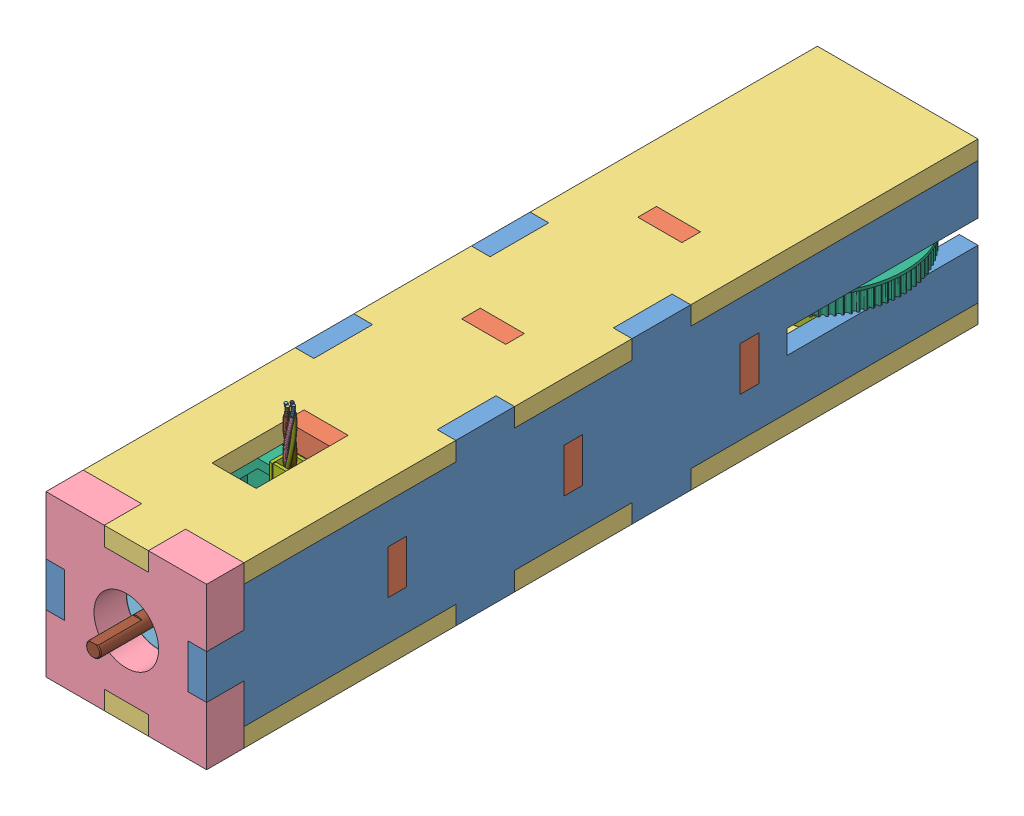
SolidWorks assembly AssemV2, configuration Default. Lengths in mm.
Overall size (62 66.35 283.73).
31 component instances, 25 part files, 21 mates.
Components (placement in the parent):
- sideTop-1: sideTop [Default] at (73.9588 160.2156 190.6262) size (6.35 54.7 262.7)
- supportColonne-1: supportColonne [Default] at (101.3088 160.2156 260.2762) size (54.7 54.7 6.35)
- side-1: side [Default] at (101.3088 187.5656 190.6262) x (0 -1 0) z (0 0 1) size (6.35 54.7 262.7)
- top-1: top [Default] at (101.3088 160.2156 315.6262) size (54.7 54.7 12.7)
- NEMA17 x 48.step-1: NEMA17 x 48.step [Default] at (101.3088 160.2156 315.6262) x (1 0 0) z (0 1 0) size (42 72 60)
  - Frontplate.step-1: Frontplate.step [Défaut] at (0 10.5 0) size (42 12.5 42)
  - Backplate.step-1: Backplate.step [Défaut] at (0 48 0) size (42 10.5 42)
  - Connenctor.step-1: Connenctor.step [Défaut] at (0 39.5 22) size (7 7 7)
  - Housing.step-1: Housing.step [Défaut] at (0 7.5 0) size (42 17 42)
  - Bearing dummy.step-1: Bearing dummy.step [Défaut] at (0 4 0) size (22 7 22)
  - Bearing dummy 01.step-1: Bearing dummy 01.step [Défaut] at (0 43 0) size (22 7 22)
  - Core.step-1: Core.step [Défaut] at origin size (30 55.5 30)
  - M3x40-Screw.step-1: M3x40-Screw.step [Default] at (15.5 45.6 15.5) x (1 0 0) z (0 1 0) size (5.5 5.5 42)
  - M3x40-Screw001.step-1: M3x40-Screw001.step [Default] at (-15.5 45.6 15.5) x (1 0 0) z (0 1 0) size (5.5 5.5 42)
  - M3x40-Screw002.step-1: M3x40-Screw002.step [Default] at (-15.5 45.6 -15.5) x (1 0 0) z (0 1 0) size (5.5 5.5 42)
  - M3x40-Screw003.step-1: M3x40-Screw003.step [Default] at (15.5 45.6 -15.5) x (1 0 0) z (0 1 0) size (5.5 5.5 42)
  - Cable-1of4.step-1: Cable-1of4.step [Défaut] at (0 43 0) size (3.44 3.69 21)
  - Copper-1of4.step-1: Copper-1of4.step [Défaut] at (0 43 0) size (2.77 3.05 24)
  - Cable-2of4.step-1: Cable-2of4.step [Défaut] at (0 43 0) x (0 1 0) z (0 0 1) size (3.44 3.69 21)
  - Copper-4of4.step-1: Copper-4of4.step [Défaut] at (0 43 0) x (0 -1 0) z (0 0 1) size (2.77 3.05 24)
  - Cable-3of4.step-1: Cable-3of4.step [Défaut] at (0 43 0) x (-1 0 0) z (0 0 1) size (3.44 3.69 21)
  - Copper-3of4.step-1: Copper-3of4.step [Défaut] at (0 43 0) x (-1 0 0) z (0 0 1) size (2.77 3.05 24)
  - Cable-4of4.step-1: Cable-4of4.step [Défaut] at (0 43 0) x (0 -1 0) z (0 0 1) size (3.44 3.69 21)
  - Copper-2of4.step-1: Copper-2of4.step [Défaut] at (0 43 0) x (0 1 0) z (0 0 1) size (2.77 3.05 24)
- sideTop-3: sideTop [Default] at (122.3088 160.2156 190.6262) size (6.35 54.7 262.7)
- supportColonne-2: supportColonne [Default] at (101.3088 160.2156 200.2762) size (54.7 54.7 6.35)
- supportColonne-3: supportColonne [Default] at (101.3088 160.2156 140.2762) size (54.7 54.7 6.35)
- poulieV3-1: poulieV3 [Výchozí] at (100.6518 160.2156 93.5959) size (62 8 62)
- 7806K755_Thrust Ball Bearing-1: 7806K755_Thrust Ball Bearing [7806K755] at (100.6895 146.2156 83.9195) x (0.795952 0 0.60536) z (-0.60536 0 0.795952) size (40 14 40)
- 7806K755_Thrust Ball Bearing-2: 7806K755_Thrust Ball Bearing [7806K755] at (100.9459 174.2156 91.0306) x (0.507264 0 0.86179) z (0.86179 0 -0.507264) size (40 14 40)
- side-3: side [Default] at (101.3088 139.2156 190.6262) x (0 -1 0) z (0 0 1) size (6.35 54.7 262.7)
Mates (geometry in assembly coordinates):
- Coincident2: coincident aligned: plane of sideTop-1 through (80.3088 160.2156 328.3262) normal (0 0 1); plane of top-1 through (101.3088 160.2156 328.3262) normal (0 0 1)
- Coincident6: coincident anti-aligned: plane of sideTop-1 through (80.3088 160.2156 190.6262) normal (1 0 0); plane of top-1 through (80.3088 152.7156 315.6262) normal (-1 0 0)
- Coincident7: coincident anti-aligned: plane of sideTop-1 through (80.3088 167.7156 190.6262) normal (0 1 0); plane of top-1 through (73.9588 167.7156 315.6262) normal (0 -1 0)
- Coincident8: coincident aligned: plane of sideTop-1 through (73.9588 160.2156 190.6262) normal (-1 0 0); plane of supportColonne-1 through (73.9588 132.8656 266.6262) normal (-1 0 0)
- Coincident9: coincident anti-aligned: plane of sideTop-1 through (73.9588 167.7156 260.2762) normal (0 -1 0); plane of supportColonne-1 through (101.3088 167.7156 260.2762) normal (0 1 0)
- Coincident10: coincident anti-aligned: plane of sideTop-1 through (73.9588 152.7156 266.6262) normal (0 0 -1); plane of supportColonne-1 through (101.3088 160.2156 266.6262) normal (0 0 1)
- Concentric1: concentric aligned: circle of top-1; circle of NEMA17 x 48.step-1/Frontplate.step-1
- Coincident11: coincident anti-aligned: plane of top-1 through (101.3088 160.2156 315.6262) normal (0 0 -1); plane of NEMA17 x 48.step-1/Frontplate.step-1 through (101.3088 160.2156 315.6262) normal (0 0 1)
- Coincident12: coincident aligned: plane of top-1 through (93.8088 181.2156 315.6262) normal (0 1 0); plane of NEMA17 x 48.step-1/Frontplate.step-1 through (118.2793 181.2156 305.1262) normal (0 1 0)
- Coincident13: coincident anti-aligned: plane of side-1 through (101.3088 181.2156 190.6262) normal (0 -1 0); plane of top-1 through (93.8088 181.2156 315.6262) normal (0 1 0)
- Coincident14: coincident anti-aligned: plane of side-1 through (108.8088 181.2156 190.6262) normal (1 0 0); plane of top-1 through (108.8088 187.5656 315.6262) normal (-1 0 0)
- Coincident15: coincident aligned: plane of side-1 through (101.3088 181.2156 328.3262) normal (0 0 1); plane of top-1 through (101.3088 160.2156 328.3262) normal (0 0 1)
- Coincident16: coincident aligned: plane of sideTop-1 through (73.9588 160.2156 190.6262) normal (-1 0 0); plane of supportColonne-2 through (73.9588 132.8656 206.6262) normal (-1 0 0)
- Coincident17: coincident aligned: plane of sideTop-1 through (80.3088 139.2156 190.6262) normal (0 -1 0); plane of supportColonne-2 through (101.3088 139.2156 200.2762) normal (0 -1 0)
- Coincident18: coincident anti-aligned: plane of sideTop-1 through (73.9588 152.7156 206.6262) normal (0 0 -1); plane of supportColonne-2 through (101.3088 160.2156 206.6262) normal (0 0 1)
- Coincident19: coincident anti-aligned: plane of sideTop-1 through (73.9588 152.7156 140.2762) normal (0 0 1); plane of supportColonne-3 through (101.3088 160.2156 140.2762) normal (0 0 -1)
- Coincident20: coincident aligned: plane of sideTop-1 through (73.9588 160.2156 190.6262) normal (-1 0 0); plane of supportColonne-3 through (73.9588 132.8656 146.6262) normal (-1 0 0)
- Coincident21: coincident anti-aligned: plane of sideTop-1 through (73.9588 152.7156 140.2762) normal (0 1 0); plane of supportColonne-3 through (101.3088 152.7156 140.2762) normal (0 -1 0)
- Coincident22: coincident anti-aligned: plane of sideTop-3 through (122.3088 164.2156 65.6262) normal (0 -1 0); plane of poulieV3-1 through (100.6518 164.2156 93.5959) normal (0 1 0)
- Coincident23: coincident anti-aligned: plane of side-1 through (101.3088 181.2156 190.6262) normal (0 -1 0); plane of 7806K755_Thrust Ball Bearing-2 through (95.8023 181.2156 82.292) normal (0 1 0)
- Coincident24: coincident anti-aligned: plane of 7806K755_Thrust Ball Bearing-1 through (92.6185 139.2156 77.7812) normal (0 -1 0); plane of side-3 through (101.3088 139.2156 190.6262) normal (0 1 0)
